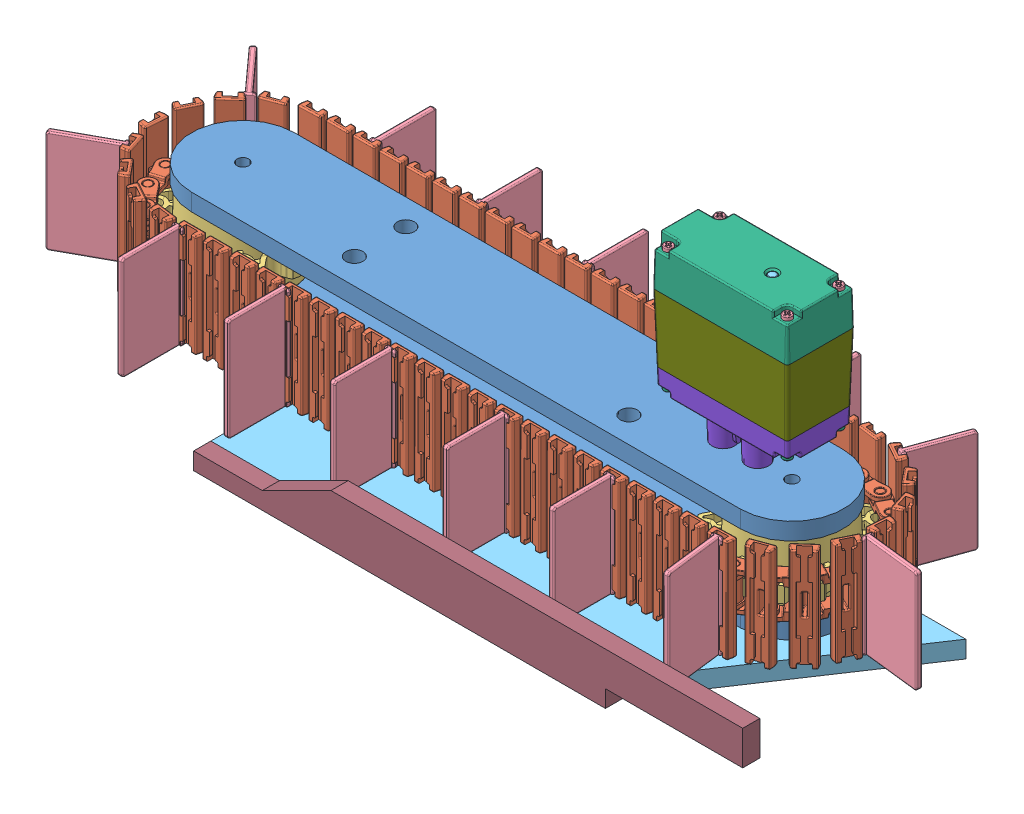
SolidWorks assembly CubeIntake, configuration Default. Lengths in mm.
Overall size (304.47 107.05 117.04).
116 component instances, 31 part files, 17 mates.
Components (placement in the parent):
- CubeIntakePlate-1: CubeIntakePlate [Default] at origin size (241.3 6.35 38.1)
- Base-Link-1: Base-Link [Default] at (65.3118 19.05 30.6215) x (-1 0 0) z (0 -1 0) size (16.96 9.71 38)
- sprocket-1: sprocket [Default] at (0 31.75 0) x (0.991922 0 0.126848) z (0 -1 0) size (50.77 50.68 25.4)
- sprocket-2: sprocket [Default] at (203.2 31.75 0) x (1 0 0) z (0 -1 0) size (50.77 50.68 25.4)
- CubeIntakePlate-2: CubeIntakePlate [Default] at (0 31.75 0) size (241.3 6.35 38.1)
- Base-Link-2: Base-Link [Default] at (75.1118 19.05 30.6215) x (-1 0 0) z (0 -1 0) size (16.96 9.71 38)
- Base-Link-3: Base-Link [Default] at (84.9118 19.05 30.6215) x (-1 0 0) z (0 -1 0) size (16.96 9.71 38)
- Base-Link-4: Base-Link [Default] at (94.7118 19.05 30.6215) x (-1 0 0) z (0 -1 0) size (16.96 9.71 38)
- Base-Link-5: Base-Link [Default] at (104.5118 19.05 30.6215) x (-1 0 0) z (0 -1 0) size (16.96 9.71 38)
- Base-Link-6: Base-Link [Default] at (114.3118 19.05 30.6215) x (-1 0 0) z (0 -1 0) size (16.96 9.71 38)
- Base-Link-7: Base-Link [Default] at (124.1118 19.05 30.6215) x (-1 0 0) z (0 -1 0) size (16.96 9.71 38)
- Base-Link-8: Base-Link [Default] at (133.9118 19.05 30.6215) x (-1 0 0) z (0 -1 0) size (16.96 9.71 38)
- Base-Link-9: Base-Link [Default] at (143.7118 19.05 30.6215) x (-1 0 0) z (0 -1 0) size (16.96 9.71 38)
- Base-Link-10: Base-Link [Default] at (153.5118 19.05 30.6215) x (-1 0 0) z (0 -1 0) size (16.96 9.71 38)
- Base-Link-11: Base-Link [Default] at (163.3118 19.05 30.6215) x (-1 0 0) z (0 -1 0) size (16.96 9.71 38)
- Base-Link-12: Base-Link [Default] at (173.1118 19.05 30.6215) x (-1 0 0) z (0 -1 0) size (16.96 9.71 38)
- Base-Link-13: Base-Link [Default] at (182.9118 19.05 30.6215) x (-1 0 0) z (0 -1 0) size (16.96 9.71 38)
- Base-Link-14: Base-Link [Default] at (192.7118 19.05 30.6215) x (-1 0 0) z (0 -1 0) size (16.96 9.71 38)
- Base-Link-15: Base-Link [Default] at (202.6735 19.05 30.4469) x (-0.999386 0 0.035048) z (0 -1 0) size (16.96 9.71 38)
- Base-Link-16: Base-Link [Default] at (213.6289 19.05 28.2933) x (-0.938289 0 0.345853) z (0 -1 0) size (16.96 9.71 38)
- Base-Link-17: Base-Link [Default] at (223.3874 19.05 22.3996) x (-0.742835 0 0.669474) z (0 -1 0) size (16.96 9.71 38)
- Base-Link-18: Base-Link [Default] at (230.2605 19.05 13.3042) x (-0.441206 0 0.897406) z (0 -1 0) size (16.96 9.71 38)
- Base-Link-19: Base-Link [Default] at (233.2658 19.05 2.3072) x (-0.076515 0 0.997068) z (0 -1 0) size (16.96 9.71 38)
- Base-Link-20: Base-Link [Default] at (231.9736 19.05 -9.0195) x (0.299113 0 0.954218) z (0 -1 0) size (16.96 9.71 38)
- Base-Link-21: Base-Link [Default] at (226.5688 19.05 -19.0571) x (0.631988 0 0.774978) z (0 -1 0) size (16.96 9.71 38)
- Base-Link-22: Base-Link [Default] at (217.8238 19.05 -26.3708) x (0.874532 0 0.484968) z (0 -1 0) size (16.96 9.71 38)
- Base-Link-23: Base-Link [Default] at (207.0177 19.05 -29.9386) x (0.99137 0 0.131091) z (0 -1 0) size (16.96 9.71 38)
- Base-Link-24: Base-Link [Default] at (196.6438 19.05 -30.6215) x (1 0 0) z (0 -1 0) size (16.96 9.71 38)
- Base-Link-25: Base-Link [Default] at (186.8438 19.05 -30.6215) x (1 0 0) z (0 -1 0) size (16.96 9.71 38)
- Base-Link-26: Base-Link [Default] at (177.0438 19.05 -30.6215) x (1 0 0) z (0 -1 0) size (16.96 9.71 38)
- Base-Link-27: Base-Link [Default] at (167.2438 19.05 -30.6215) x (1 0 0) z (0 -1 0) size (16.96 9.71 38)
- Base-Link-28: Base-Link [Default] at (157.4438 19.05 -30.6215) x (1 0 0) z (0 -1 0) size (16.96 9.71 38)
- Base-Link-29: Base-Link [Default] at (147.6438 19.05 -30.6215) x (1 0 0) z (0 -1 0) size (16.96 9.71 38)
- Base-Link-30: Base-Link [Default] at (137.8438 19.05 -30.6215) x (1 0 0) z (0 -1 0) size (16.96 9.71 38)
- Base-Link-31: Base-Link [Default] at (128.0438 19.05 -30.6215) x (1 0 0) z (0 -1 0) size (16.96 9.71 38)
- Base-Link-32: Base-Link [Default] at (118.2438 19.05 -30.6215) x (1 0 0) z (0 -1 0) size (16.96 9.71 38)
- Base-Link-33: Base-Link [Default] at (108.4438 19.05 -30.6215) x (1 0 0) z (0 -1 0) size (16.96 9.71 38)
- Base-Link-34: Base-Link [Default] at (98.6438 19.05 -30.6215) x (1 0 0) z (0 -1 0) size (16.96 9.71 38)
- Base-Link-35: Base-Link [Default] at (88.8438 19.05 -30.6215) x (1 0 0) z (0 -1 0) size (16.96 9.71 38)
- Base-Link-36: Base-Link [Default] at (79.0438 19.05 -30.6215) x (1 0 0) z (0 -1 0) size (16.96 9.71 38)
- Base-Link-37: Base-Link [Default] at (69.2438 19.05 -30.6215) x (1 0 0) z (0 -1 0) size (16.96 9.71 38)
- Base-Link-38: Base-Link [Default] at (59.4438 19.05 -30.6215) x (1 0 0) z (0 -1 0) size (16.96 9.71 38)
- Base-Link-39: Base-Link [Default] at (49.6438 19.05 -30.6215) x (1 0 0) z (0 -1 0) size (16.96 9.71 38)
- Base-Link-40: Base-Link [Default] at (39.8438 19.05 -30.6215) x (1 0 0) z (0 -1 0) size (16.96 9.71 38)
- Base-Link-41: Base-Link [Default] at (30.0438 19.05 -30.6215) x (1 0 0) z (0 -1 0) size (16.96 9.71 38)
- Base-Link-42: Base-Link [Default] at (20.2438 19.05 -30.6215) x (1 0 0) z (0 -1 0) size (16.96 9.71 38)
- Base-Link-43: Base-Link [Default] at (10.4438 19.05 -30.6215) x (1 0 0) z (0 -1 0) size (16.96 9.71 38)
- Base-Link-44: Base-Link [Default] at (0.4788 19.05 -30.4431) x (0.999359 0 -0.035792) z (0 -1 0) size (16.96 9.71 38)
- Base-Link-45: Base-Link [Default] at (-10.4777 19.05 -28.2753) x (0.937691 0 -0.34747) z (0 -1 0) size (16.96 9.71 38)
- Base-Link-46: Base-Link [Default] at (-20.226 19.05 -22.3647) x (0.74168 0 -0.670754) z (0 -1 0) size (16.96 9.71 38)
- Base-Link-47: Base-Link [Default] at (-27.0834 19.05 -13.2575) x (0.439659 0 -0.898165) z (0 -1 0) size (16.96 9.71 38)
- Base-Link-48: Base-Link [Default] at (-30.0697 19.05 -2.2554) x (0.074796 0 -0.997199) z (0 -1 0) size (16.96 9.71 38)
- Base-Link-49: Base-Link [Default] at (-28.758 19.05 9.0691) x (-0.300758 0 -0.953701) z (0 -1 0) size (16.96 9.71 38)
- Base-Link-50: Base-Link [Default] at (-23.3359 19.05 19.0973) x (-0.633323 0 -0.773887) z (0 -1 0) size (16.96 9.71 38)
- Base-Link-51: Base-Link [Default] at (-14.5783 19.05 26.3959) x (-0.875366 0 -0.48346) z (0 -1 0) size (16.96 9.71 38)
- Base-Link-52: Base-Link [Default] at (-3.7676 19.05 29.9464) x (-0.991556 0 -0.129677) z (0 -1 0) size (16.96 9.71 38)
- Base-Link-53: Base-Link [Default] at (6.6005 19.05 30.6215) x (-1 0 0) z (0 -1 0) size (16.96 9.71 38)
- Base-Link-54: Base-Link [Default] at (16.4005 19.05 30.6215) x (-1 0 0) z (0 -1 0) size (16.96 9.71 38)
- Base-Link-55: Base-Link [Default] at (26.2005 19.05 30.6215) x (-1 0 0) z (0 -1 0) size (16.96 9.71 38)
- Base-Link-56: Base-Link [Default] at (36.0005 19.05 30.6215) x (-1 0 0) z (0 -1 0) size (16.96 9.71 38)
- Base-Link-57: Base-Link [Default] at (45.8005 19.05 30.6215) x (-1 0 0) z (0 -1 0) size (16.96 9.71 38)
- Base-Link-58: Base-Link [Default] at (55.6005 19.05 30.6215) x (-1 0 0) z (0 -1 0) size (16.96 9.71 38)
- fin-1: fin [Default] at (128.3398 19.05 31.2392) x (-1 0 0) z (0 1 0) size (4 22.3 38)
- fin-15: fin [Default] at (167.6618 19.05 31.2392) x (-1 0 0) z (0 1 0) size (4 22.3 38)
- fin-16: fin [Default] at (206.9727 19.05 30.9743) x (-0.992664 0 0.120907) z (0 1 0) size (4 22.3 38)
- fin-17: fin [Default] at (234.2051 19.05 3.5105) x (-0.112503 0 0.993651) z (0 1 0) size (4 22.3 38)
- fin-18: fin [Default] at (213.8023 19.05 -29.3467) x (0.940504 0 0.339784) z (0 1 0) size (4 22.3 38)
- fin-19: fin [Default] at (174.5959 19.05 -31.2392) x (1 0 0) z (0 1 0) size (4 22.3 38)
- fin-20: fin [Default] at (135.2739 19.05 -31.2392) x (1 0 0) z (0 1 0) size (4 22.3 38)
- fin-21: fin [Default] at (95.9519 19.05 -31.2392) x (1 0 0) z (0 1 0) size (4 22.3 38)
- fin-22: fin [Default] at (56.6299 19.05 -31.2392) x (1 0 0) z (0 1 0) size (4 22.3 38)
- fin-23: fin [Default] at (17.3079 19.05 -31.2392) x (1 0 0) z (0 1 0) size (4 22.3 38)
- fin-24: fin [Default] at (-20.9282 19.05 -23.1441) x (0.741723 0 -0.670706) z (0 1 0) size (4 22.3 38)
- fin-25: fin [Default] at (-27.3652 19.05 14.9929) x (-0.480492 0 -0.876999) z (0 1 0) size (4 22.3 38)
- fin-26: fin [Default] at (7.9669 19.05 31.2392) x (-1 0 0) z (0 1 0) size (4 22.3 38)
- fin-27: fin [Default] at (47.2889 19.05 31.2392) x (-1 0 0) z (0 1 0) size (4 22.3 38)
- fin-28: fin [Default] at (86.6109 19.05 31.2392) x (-1 0 0) z (0 1 0) size (4 22.3 38)
- CubeIntakePlatform-1: CubeIntakePlatform [Default] at (132.3749 -6.35 24.4929) size (203.2 6.35 76.2)
- DRIVE MOTOR-1: DRIVE MOTOR [Default] at (177.5 86.1 0) size (56.4 63.4 25)
  - SPPM206-0150BO-1: SPPM206-0150BO [Default] at (-10.5 -23.5 -9.5) x (-1 0 0) z (0 0 1) size (3.3 16.36 3.3)
  - 276-2177-004 Rev1-1: 276-2177-004 Rev1 [Default] at (0 2.3 0) x (-0.521464 0 -0.853273) z (0 -1 0) size (5.83 5.83 4.5)
  - 276-2177-003 Rev1-1: 276-2177-003 Rev1 [Default] at (0 -25 0) size (48.69 26 23.69)
  - SPPM204-0050BO-1: SPPM204-0050BO [Default] at (0 -6.45 -6.2) size (3.3 6.41 3.3)
  - 276-2177-014 Rev1-1: 276-2177-014 Rev1 [Default] at (-11.6 -15 0) x (0 1 0) z (0 0 1) size (1 18.4 20.4)
  - 276-2177-005 Rev1-1: 276-2177-005 Rev1 [Default] at (12.1 2.15 0) x (-0.981818 0 0.189823) z (0 -1 0) size (19.95 19.95 7)
  - 276-2177-015 Rev2-1: 276-2177-015 Rev2 [Default] at (15.1 -10.55 0) x (-0.403604 0 0.914934) z (0 -1 0) size (14.01 14.03 13)
  - SPPM206-0150BO-2: SPPM206-0150BO [Default] at (33.5 -23.5 9.5) x (-1 0 0) z (0 0 1) size (3.3 16.36 3.3)
  - 276-2177-019 Rev1-1: 276-2177-019 Rev1 [Default] at (13 -33 0) x (0.158525 0 -0.987355) z (-0.987355 0 -0.158525) size (6.3 15.8 6.3)
  - 276-2177-016 Rev2-1: 276-2177-016 Rev2 [Default] at (25.7 -19.25 0) x (-0.479705 0 -0.87743) z (0 -1 0) size (15.08 15.08 17.5)
  - 276-2177-012 Rev1-1: 276-2177-012 Rev1 [Default] at (25.7 -19.1 0) x (-0.525336 0 0.850895) z (0 1 0) size (6 6 2.85)
  - 276-2177-002 Rev1-1: 276-2177-002 Rev1 [Default] at origin size (50 27.05 25)
  - LABLE_1-1: LABLE_1 [Default] at (27.1066 -2.1 2.9971) x (0.995174 0 0.098129) z (0 1 0) size (12 12 0.21)
  - 276-2177-011 Rev1-1: 276-2177-011 Rev1 [Default] at (12.1 -0.9 0) x (0 1 0) z (-0.101873 0 0.994797) size (14.8 2 2)
  - SPPM204-0050BO-2: SPPM204-0050BO [Default] at (0 -6.45 6.2) size (3.3 6.41 3.3)
  - FS130-FT-21100-1: FS130-FT-21100 [Default] at (0 -15 0) x (0 0 -1) z (0 1 0) size (20.4 15.4 34.7)
  - 276-2177-010 Rev1-1: 276-2177-010 Rev1 [Default] at (24.2 -4.9 0) x (0 1 0) z (0.653198 0 -0.757187) size (20.8 2 2)
  - 276-2177-006 Rev1-1: 276-2177-006 Rev1 [Default] at (24.2 -0.95 0) x (-0.999044 0 -0.043716) z (0 -1 0) size (20.25 20.26 13)
  - 276-1321-INST1-1: 276-1321-INST1 [Default] at origin size (52.31 18.11 25)
    - M2_1-1: M2_1 [Default] at (33.5 5 9.5) size (3.3 17.41 3.3)
    - LIGHT_1-1: LIGHT_1 [Default] at (-1.2 -1.6 0) x (-1 0 0) z (0 1 0) size (4.3 7.9 4.5)
    - M2_1-2: M2_1 [Default] at (-10.5 5 -9.5) size (3.3 17.41 3.3)
    - BOX-BOTTOM2_3-1: BOX-BOTTOM2_3 [Default] at origin size (52.31 14.6 25)
    - M2_1-3: M2_1 [Default] at (-10.5 5 9.5) size (3.3 17.41 3.3)
    - LABLE_1-1: LABLE_1 [Default] at (-3.1282 -2.1 -1.5101) x (-1 0 0) z (0 1 0) size (12 12 0.21)
    - M2_1-4: M2_1 [Default] at (33.5 5 -9.5) size (3.3 17.41 3.3)
    - PCB2_3-1: PCB2_3 [Default] at origin size (35.5 5.9 20)
    - PIN_ASM_1_ASM-1: PIN_ASM_1_ASM [Default] at (-2 9.01 -0.5) x (0 1 0) z (0 0 1) size (7.84 15.75 10.2)
      - PIN2_1-1: PIN2_1 [Default] at (2.62 -5.9 0) size (7.74 10.15 10.2)
      - PIN_1-1: PIN_1 [Default] at origin size (5.2 9.95 10.2)
  - 276-2177-019 Rev1-2: 276-2177-019 Rev1 [Default] at (0.3 -33 0) x (-0.999228 0 0.03928) z (0.03928 0 0.999228) size (6.3 15.8 6.3)
  - 276-2177-018 Rev1-1: 276-2177-018 Rev1 [Default] at (-12 2.1 0) x (0 0 -1) z (1 0 0) size (6.41 4.2 8.9)
  - SPPM206-0150BO-3: SPPM206-0150BO [Default] at (33.5 -23.5 -9.5) x (-1 0 0) z (0 0 1) size (3.3 16.36 3.3)
  - 276-2177-013 Rev1-1: 276-2177-013 Rev1 [Default] at (25.7 -31.5 0) x (-1 0 0) z (0 1 0) size (10 9.93 10.05)
  - SPPM206-0150BO-4: SPPM206-0150BO [Default] at (-10.5 -23.5 9.5) x (-1 0 0) z (0 0 1) size (3.3 16.36 3.3)
  - 276-2177-009 Rev1-1: 276-2177-009 Rev1 [Default] at (15.1 -17.75 0) x (1 0 0) z (0 -1 0) size (2 2 27.5)
- CubeIntakeSupport-2: CubeIntakeSupport [Default] at (45.2892 -6.35 57.15) x (0 0 -1) z (1 0 0) size (6.35 19.05 203.2)
Mates (geometry in assembly coordinates):
- Coincident1: coincident anti-aligned: plane of CubeIntakePlate-1 through (0 6.35 0) normal (0 1 0); plane of sprocket-1 through (0 6.35 0) normal (0 -1 0)
- Coincident2: coincident anti-aligned: plane of CubeIntakePlate-1 through (0 6.35 0) normal (0 1 0); plane of sprocket-2 through (203.2 6.35 0) normal (0 -1 0)
- Concentric1: concentric aligned: circle of CubeIntakePlate-1; circle of sprocket-1
- Concentric2: concentric aligned: circle of CubeIntakePlate-1; circle of sprocket-2
- Concentric3: concentric aligned: cylinder of CubeIntakePlate-1 through (203.2 6.35 0) axis (0 -1 0) radius 2.1828; cylinder of CubeIntakePlate-2 through (203.2 38.1 0) axis (0 -1 0) radius 2.1828
- Concentric4: concentric aligned: cylinder of CubeIntakePlate-1 through (0 6.35 0) axis (0 -1 0) radius 2.1828; cylinder of CubeIntakePlate-2 through (0 38.1 0) axis (0 -1 0) radius 2.1828
- Coincident3: coincident anti-aligned: plane of sprocket-1 through (0 31.75 0) normal (0 1 0); plane of CubeIntakePlate-2 through (0 31.75 0) normal (0 -1 0)
- GearMate1: gear = 5 : 5.08 mm: cone of sprocket-1 through (0 19.8 0) axis (0 1 0); cylinder of Base-Link-14 through (197.6118 15.05 25.9215) axis (0 -1 0) radius 2.5
- Lock3: lock: unknown of Base-Link-13; unknown of fin-1
- Coincident11: coincident anti-aligned: plane of CubeIntakePlate-1 through (0 0 0) normal (0 -1 0); plane of CubeIntakePlatform-1 through (132.3749 0 24.4929) normal (0 1 0)
- Concentric6: concentric aligned: cylinder of CubeIntakePlate-1 through (152.4 6.35 -9.525) axis (0 -1 0) radius 3.175; cylinder of CubeIntakePlatform-1 through (152.4 0 -9.525) axis (0 -1 0) radius 3.175
- Concentric7: concentric aligned: cylinder of CubeIntakePlate-1 through (152.4 6.35 9.525) axis (0 -1 0) radius 3.175; cylinder of CubeIntakePlatform-1 through (152.4 0 9.525) axis (0 -1 0) radius 3.175
- Coincident13: coincident aligned: plane of CubeIntakePlate-2 through (0 38.1 0) normal (0 1 0); circle of DRIVE MOTOR-1/276-2177-003 Rev1-1
- Concentric9: concentric aligned: circle of CubeIntakePlate-2; circle of DRIVE MOTOR-1/276-2177-003 Rev1-1
- Parallel4: parallel aligned: line of CubeIntakePlate-2 through (203.2 38.1 -19.05) axis (-1 0 0); line of DRIVE MOTOR-1/276-1321-INST1-1/BOX-BOTTOM2_3-1 through (213 86.1 -12.5) axis (-1 0 0)
- Coincident16: coincident aligned: line of CubeIntakePlatform-1 through (197.6892 0 57.15) axis (0 -1 0); line of CubeIntakeSupport-2 through (197.6892 0 57.15) axis (0 -1 0)
- Coincident17: coincident anti-aligned: line of CubeIntakePlatform-1 through (45.2892 -6.35 57.15) axis (1 0 0); line of CubeIntakeSupport-2 through (197.6892 -6.35 57.15) axis (-1 0 0)
